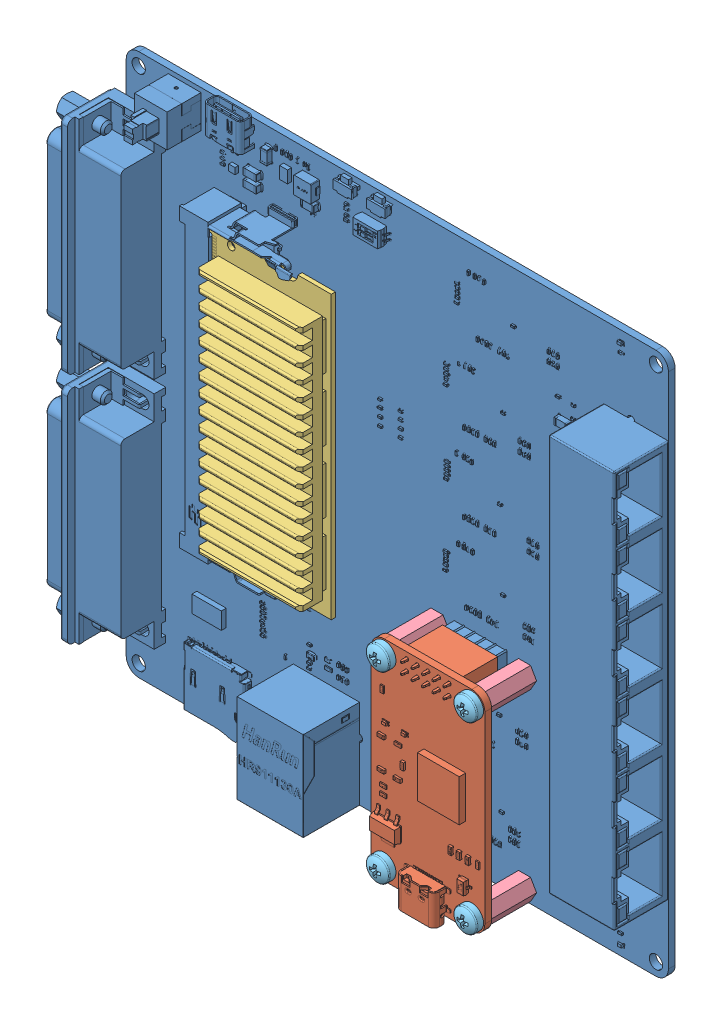
SolidWorks assembly OECU, configuration 默认. Lengths in mm.
Overall size (138.75 131.78 21.94).
15 component instances, 5 part files, 29 mates.
Components (placement in the parent):
- OECU_BASE-1: OECU_BASE [默认] at (-88.4612 -71.2683 135.0327) size (138.75 130.63 19.64)
- MY_JATG-1: MY_JATG [默认] at (0.4762 -34.5435 96.6573) x (-1 0 0) z (0 0 1) size (27.25 51.32 13.3)
- ZYNQ_CORE-1: ZYNQ_CORE [1.5V] at (-51.5412 15.3817 142.3027) x (0 -1 0) z (-1 0 0) size (67.6 9 30)
- Column_M3x11-1: Column_M3x11 [Predeterminado] at (-3.9592 -58.2563 141.0327) x (1 0 0) z (0 -1 0) size (5.77 11 5)
- Column_M3x11-2: Column_M3x11 [Predeterminado] at (17.0408 -58.2563 141.0327) x (1 0 0) z (0 -1 0) size (5.77 11 5)
- Column_M3x11-3: Column_M3x11 [Predeterminado] at (-3.9592 -14.2563 141.0327) x (1 0 0) z (0 -1 0) size (5.77 11 5)
- Column_M3x11-4: Column_M3x11 [Predeterminado] at (17.0408 -14.2563 141.0327) x (1 0 0) z (0 -1 0) size (5.77 11 5)
- Bolt_M3x6-1: Bolt_M3x6 [B18.6.7M - M3 x 0.5 x 6 Type I Cross Recessed PHMS --6N] at (-3.9592 -58.2563 150.0727) x (0 0 -1) z (1 0 0) size (8.37 5.6 5.6)
- Bolt_M3x6-2: Bolt_M3x6 [B18.6.7M - M3 x 0.5 x 6 Type I Cross Recessed PHMS --6N] at (-3.9592 -14.2563 131.0291) x (0 0 1) z (-0.992533 -0.121977 0) size (8.37 5.6 5.6)
- Bolt_M3x6-3: Bolt_M3x6 [B18.6.7M - M3 x 0.5 x 6 Type I Cross Recessed PHMS --6N] at (17.0408 -58.2563 131.0291) x (0 0 1) z (-0.983022 0.183489 0) size (8.37 5.6 5.6)
- Bolt_M3x6-4: Bolt_M3x6 [B18.6.7M - M3 x 0.5 x 6 Type I Cross Recessed PHMS --6N] at (-3.9592 -58.2563 131.0291) x (0 0 1) z (-0.995776 -0.091819 0) size (8.37 5.6 5.6)
- Bolt_M3x6-5: Bolt_M3x6 [B18.6.7M - M3 x 0.5 x 6 Type I Cross Recessed PHMS --6N] at (17.0408 -14.2563 131.0291) x (0 0 1) z (-0.999148 0.041272 0) size (8.37 5.6 5.6)
- Bolt_M3x6-6: Bolt_M3x6 [B18.6.7M - M3 x 0.5 x 6 Type I Cross Recessed PHMS --6N] at (17.0408 -58.2563 150.0727) x (0 0 -1) z (1 0 0) size (8.37 5.6 5.6)
- Bolt_M3x6-7: Bolt_M3x6 [B18.6.7M - M3 x 0.5 x 6 Type I Cross Recessed PHMS --6N] at (17.0408 -14.2563 150.0727) x (0 0 -1) z (1 0 0) size (8.37 5.6 5.6)
- Bolt_M3x6-8: Bolt_M3x6 [B18.6.7M - M3 x 0.5 x 6 Type I Cross Recessed PHMS --6N] at (-3.9592 -14.2563 150.0727) x (0 0 -1) z (1 0 0) size (8.37 5.6 5.6)
Mates (geometry in assembly coordinates):
- 重合1: coincident anti-aligned: plane of OECU_BASE-1 through (11.6188 -13.8843 137.5727) normal (0 0 1); plane of MY_JATG-1 through (13.1388 -11.3443 137.5727) normal (0 0 -1)
- 重合2: coincident aligned: plane of OECU_BASE-1 through (5.0148 -11.3443 135.0327) normal (0 1 0); plane of MY_JATG-1 through (13.1388 -11.3443 146.0727) normal (0 1 0)
- 距离1: distance = 0.25 mm aligned: plane of OECU_BASE-1 through (0.1888 -13.8843 137.5727) normal (-1 0 0); plane of MY_JATG-1 through (-0.0612 -13.8443 146.0727) normal (-1 0 0)
- 重合4: coincident: plane of OECU_BASE-1 through (-49.7612 -20.1683 141.8027) normal (0 0 1); plane of ZYNQ_CORE-1 through (-21.5412 49.1817 141.8027) normal (0 0 -1)
- 重合5: coincident anti-aligned: plane of OECU_BASE-1 through (-49.6112 23.8817 139.6827) normal (0 -1 0); plane of ZYNQ_CORE-1 through (-51.5412 23.8817 141.8027) normal (0 1 0)
- 重合6: coincident anti-aligned: plane of OECU_BASE-1 through (-75.4612 -61.2683 135.0327) normal (0 0 1); plane of Column_M3x11-4 through (17.0408 -14.2563 135.0327) normal (0 0 -1)
- 同心1: concentric aligned: circle of MY_JATG-1; circle of Column_M3x11-4
- 重合7: coincident anti-aligned: plane of OECU_BASE-1 through (-75.4612 -61.2683 135.0327) normal (0 0 1); plane of Column_M3x11-3 through (-3.9592 -14.2563 135.0327) normal (0 0 -1)
- 同心2: concentric aligned: cylinder of MY_JATG-1 through (-3.9592 -14.2563 146.0727) axis (0 0 -1) radius 1.6; cylinder of Column_M3x11-3 through (-3.9592 -14.2563 147.0327) axis (0 0 -1) radius 1.5
- 重合8: coincident: plane of OECU_BASE-1 through (-75.4612 -61.2683 135.0327) normal (0 0 1); line of Column_M3x11-2 through (19.9275 -58.2563 135.0327) axis (-0.5 0.866025 0)
- 同心3: concentric aligned: cylinder of MY_JATG-1 through (17.0408 -58.2563 146.0727) axis (0 0 -1) radius 1.6; cylinder of Column_M3x11-2 through (17.0408 -58.2563 147.0327) axis (0 0 -1) radius 1.5
- 重合9: coincident anti-aligned: plane of OECU_BASE-1 through (-75.4612 -61.2683 135.0327) normal (0 0 1); plane of Column_M3x11-1 through (-3.9592 -58.2563 135.0327) normal (0 0 -1)
- 同心4: concentric aligned: cylinder of MY_JATG-1 through (-3.9592 -58.2563 146.0727) axis (0 0 -1) radius 1.6; cylinder of Column_M3x11-1 through (-3.9592 -58.2563 147.0327) axis (0 0 -1) radius 1.5
- 同心5: concentric aligned: cylinder of Column_M3x11-1 through (-3.9592 -58.2563 147.0327) axis (0 0 -1) radius 1.5; cylinder of Bolt_M3x6-4 through (-3.9592 -58.2563 105.6291) axis (0 0 -1) radius 1.5
- 同心6: concentric aligned: cylinder of Column_M3x11-2 through (17.0408 -58.2563 147.0327) axis (0 0 -1) radius 1.5; cylinder of Bolt_M3x6-3 through (17.0408 -58.2563 105.6291) axis (0 0 -1) radius 1.5
- 同心7: concentric aligned: cylinder of Column_M3x11-4 through (17.0408 -14.2563 147.0327) axis (0 0 -1) radius 1.5; cylinder of Bolt_M3x6-5 through (17.0408 -14.2563 105.6291) axis (0 0 -1) radius 1.5
- 同心8: concentric aligned: cylinder of Column_M3x11-3 through (-3.9592 -14.2563 147.0327) axis (0 0 -1) radius 1.5; cylinder of Bolt_M3x6-2 through (-3.9592 -14.2563 105.6291) axis (0 0 -1) radius 1.5
- 重合10: coincident anti-aligned: plane of OECU_BASE-1 through (-75.4612 -61.2683 133.4291) normal (0 0 -1); plane of Bolt_M3x6-4 through (-4.0969 -56.7627 133.4291) normal (0 0 1)
- 重合11: coincident anti-aligned: plane of OECU_BASE-1 through (-75.4612 -61.2683 133.4291) normal (0 0 -1); plane of Bolt_M3x6-3 through (17.316 -56.7818 133.4291) normal (0 0 1)
- 重合12: coincident aligned: plane of OECU_BASE-1 through (-75.4612 -61.2683 133.4291) normal (0 0 -1); circle of Bolt_M3x6-2
- 重合13: coincident aligned: plane of OECU_BASE-1 through (-75.4612 -61.2683 133.4291) normal (0 0 -1); circle of Bolt_M3x6-5
- 同心9: concentric: line of assembly; cylinder of assembly; axis of MY_JATG-1 through (-3.9592 -58.2563 147.6727) axis (0 0 -1); cylinder of Bolt_M3x6-1 through (-3.9592 -58.2563 158.1408) axis (0 0 1) radius 1.5
- 同心10: concentric: line of assembly; cylinder of assembly; axis of MY_JATG-1 through (17.0408 -58.2563 147.6727) axis (0 0 -1); cylinder of Bolt_M3x6-6 through (17.0408 -58.2563 154.1458) axis (0 0 1) radius 1.5
- 同心12: concentric anti-aligned: cylinder of MY_JATG-1 through (17.0408 -14.2563 146.0727) axis (0 0 -1) radius 1.6; cylinder of Bolt_M3x6-7 through (17.0408 -14.2563 175.4727) axis (0 0 1) radius 1.5
- 同心14: concentric anti-aligned: cylinder of MY_JATG-1 through (-3.9592 -14.2563 146.0727) axis (0 0 -1) radius 1.6; cylinder of Bolt_M3x6-8 through (-3.9592 -14.2563 175.4727) axis (0 0 1) radius 1.5
- 重合14: coincident aligned: plane of MY_JATG-1 through (17.0408 -11.1293 147.6727) normal (0 0 1); circle of Bolt_M3x6-8
- 重合15: coincident aligned: plane of MY_JATG-1 through (17.0408 -11.1293 147.6727) normal (0 0 1); circle of Bolt_M3x6-7
- 重合16: coincident aligned: plane of MY_JATG-1 through (17.0408 -11.1293 147.6727) normal (0 0 1); circle of Bolt_M3x6-6
- 重合17: coincident aligned: plane of MY_JATG-1 through (17.0408 -11.1293 147.6727) normal (0 0 1); circle of Bolt_M3x6-1
